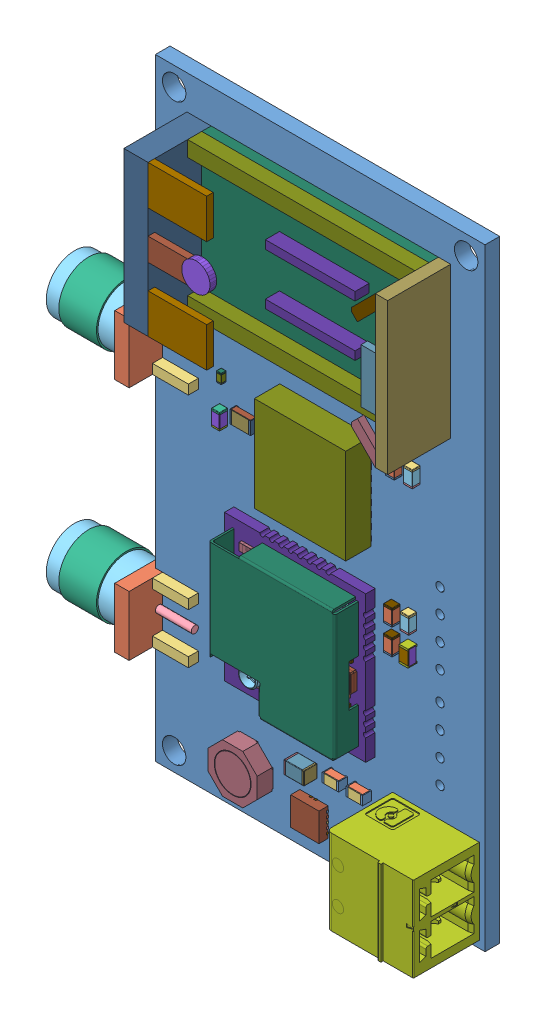
SolidWorks assembly Peggy Tracker, configuration По умолчанию. Lengths in mm.
Overall size (43.58 65 10.65).
318 component instances, 80 part files, 0 mates.
Components (placement in the parent):
- Peggy Tracker.step-1: Peggy Tracker.step [Default] at origin size (43.58 65 10.65)
  - Board.step-1: Board.step [Default] at origin size (35 65 1.56)
    - Open CASCADE STEP translator 6.8 1.1.1.step-1: Open CASCADE STEP translator 6.8 1.1.1.step [Default] at (0 0 -1.5596) size (35 65 1.56)
  - XS2.step-1: XS2.step [Default] at origin size (13.15 6.35 6.72)
    - 6208988928.step-1: 6208988928.step [Default] at (0 14.605 -2.8) size (1.52 6.35 6.35)
      - Extruded.step-1: Extruded.step [Default] at origin size (1.52 6.35 6.35)
    - 6208988528.step-1: 6208988528.step [Default] at (2.667 11.938 0) size (3.81 1.02 1.07)
      - Extruded-0.step-1: Extruded-0.step [Default] at origin size (3.81 1.02 1.07)
    - 6208988528.step-2: 6208988528.step [Default] at (2.667 17.272 0) size (3.81 1.02 1.07)
      - Extruded-0.step-1: Extruded-0.step [Default] at origin size (3.81 1.02 1.07)
    - 6208987888.step-1: 6208987888.step [Default] at (0.7603 14.6035 0.38) x (0 1 0) z (1 0 0) size (0.76 0.76 3.81)
      - Cylinder.step-1: Cylinder.step [Default] at origin size (0.76 0.76 3.81)
    - 6208988528.step-3: 6208988528.step [Default] at (2.667 11.938 -2.8) size (3.81 1.02 1.07)
      - Extruded-0.step-1: Extruded-0.step [Default] at origin size (3.81 1.02 1.07)
    - 6208988528.step-4: 6208988528.step [Default] at (2.667 17.272 -2.8) size (3.81 1.02 1.07)
      - Extruded-0.step-1: Extruded-0.step [Default] at origin size (3.81 1.02 1.07)
    - 6208987088.step-1: 6208987088.step [Default] at (-8.58 14.6049 0) x (0 1 0) z (1 0 0) size (6 6 7.87)
      - Cylinder-1.step-1: Cylinder-1.step [Default] at origin size (6 6 7.87)
    - 6208986608.step-1: 6208986608.step [Default] at (-7.0799 14.6099 0) x (0 1 0) z (1 0 0) size (6.34 6.34 4)
      - Cylinder-2.step-1: Cylinder-2.step [Default] at origin size (6.34 6.34 4)
  - XS1.step-1: XS1.step [Default] at origin size (13.15 6.35 6.72)
    - 6208986608.step-1: 6208986608.step [Default] at (-7.0799 39.6797 0) x (0 1 0) z (1 0 0) size (6.34 6.34 4)
      - Cylinder-2.step-1: Cylinder-2.step [Default] at origin size (6.34 6.34 4)
    - 6208987088.step-1: 6208987088.step [Default] at (-8.58 39.6747 0) x (0 1 0) z (1 0 0) size (6 6 7.87)
      - Cylinder-1.step-1: Cylinder-1.step [Default] at origin size (6 6 7.87)
    - 6208988528.step-1: 6208988528.step [Default] at (2.667 42.3418 -2.8) size (3.81 1.02 1.07)
      - Extruded-0.step-1: Extruded-0.step [Default] at origin size (3.81 1.02 1.07)
    - 6208988528.step-2: 6208988528.step [Default] at (2.667 37.0078 -2.8) size (3.81 1.02 1.07)
      - Extruded-0.step-1: Extruded-0.step [Default] at origin size (3.81 1.02 1.07)
    - 6208987888.step-1: 6208987888.step [Default] at (0.7603 39.6733 0.38) x (0 1 0) z (1 0 0) size (0.76 0.76 3.81)
      - Cylinder.step-1: Cylinder.step [Default] at origin size (0.76 0.76 3.81)
    - 6208988528.step-3: 6208988528.step [Default] at (2.667 42.3418 0) size (3.81 1.02 1.07)
      - Extruded-0.step-1: Extruded-0.step [Default] at origin size (3.81 1.02 1.07)
    - 6208988528.step-4: 6208988528.step [Default] at (2.667 37.0078 0) size (3.81 1.02 1.07)
      - Extruded-0.step-1: Extruded-0.step [Default] at origin size (3.81 1.02 1.07)
    - 6208988928.step-1: 6208988928.step [Default] at (0 39.6748 -2.8) size (1.52 6.35 6.35)
      - Extruded.step-1: Extruded.step [Default] at origin size (1.52 6.35 6.35)
  - X3.step-1: X3.step [Default] at origin size (9.3 9.01 10.65)
    - 1803277.step-1: 1803277.step [Default] at (25.1905 3.3527 0) x (1 0 0) z (0 -1 0) size (9.3 10.65 9.01)
  - X1.step-1: X1.step [Default] at origin size (28 16 6.7)
    - 6208991008.step-1: 6208991008.step [Default] at (11.004 53.3908 6) size (3 3 0.7)
      - Extruded-3.step-1: Extruded-3.step [Default] at origin size (3 3 0.7)
    - 6208986048.step-1: 6208986048.step [Default] at (9.0355 47.4853 6) size (6.22 4.19 0.7)
      - Extruded-4.step-1: Extruded-4.step [Default] at origin size (6.22 4.19 0.7)
    - 6208986048.step-2: 6208986048.step [Default] at (9.0355 59.2953 6) size (6.22 4.19 0.7)
      - Extruded-4.step-1: Extruded-4.step [Default] at origin size (6.22 4.19 0.7)
    - 6208985488.step-1: 6208985488.step [Default] at (4.639 53.3903 0) size (2.57 16 6.7)
      - Extruded-5.step-1: Extruded-5.step [Default] at origin size (2.57 16 6.7)
    - 6208985328.step-1: 6208985328.step [Default] at (8.0358 53.4043 6) size (4.22 2.41 0.7)
      - Extruded-6.step-1: Extruded-6.step [Default] at origin size (4.22 2.41 0.7)
    - 6208984928.step-1: 6208984928.step [Default] at (30.7032 53.3903 0) size (1.3 16 6.7)
      - Extruded-7.step-1: Extruded-7.step [Default] at origin size (1.3 16 6.7)
    - 6208984448.step-1: 6208984448.step [Default] at (28.7845 47.1665 6) size (2.54 3.55 0.7)
      - Extruded-8.step-1: Extruded-8.step [Default] at origin size (2.54 3.55 0.7)
    - 6208984128.step-1: 6208984128.step [Default] at (29.2922 53.0733 6) size (1.52 5.71 0.7)
      - Extruded-9.step-1: Extruded-9.step [Default] at origin size (1.52 5.71 0.7)
    - 6208983808.step-1: 6208983808.step [Default] at (17.9894 53.3903 0) size (24.13 16 1)
      - Extruded-10.step-1: Extruded-10.step [Default] at origin size (24.13 16 1)
    - 6208983328.step-1: 6208983328.step [Default] at (17.989 60.5658 0) size (24.13 1.65 2.5)
      - Extruded-11.step-1: Extruded-11.step [Default] at origin size (24.13 1.65 2.5)
    - 6208983328.step-2: 6208983328.step [Default] at (17.9896 46.2145 0) size (24.13 1.65 2.5)
      - Extruded-11.step-1: Extruded-11.step [Default] at origin size (24.13 1.65 2.5)
    - 6208989168.step-1: 6208989168.step [Default] at (18.9415 50.4071 0) size (9.53 0.89 2.5)
      - Extruded-12.step-1: Extruded-12.step [Default] at origin size (9.53 0.89 2.5)
    - 6208989168.step-2: 6208989168.step [Default] at (18.9415 55.8681 0) size (9.53 0.89 2.5)
      - Extruded-12.step-1: Extruded-12.step [Default] at origin size (9.53 0.89 2.5)
    - 6208982368.step-1: 6208982368.step [Default] at (28.7842 59.6128 6) size (2.54 3.55 0.7)
      - Extruded-13.step-1: Extruded-13.step [Default] at origin size (2.54 3.55 0.7)
  - R5.step-1: R5.step [Default] at origin size (1.75 0.95 0.95)
    - 6200588496.step-1: 6200588496.step [Default] at (19.5326 8.3312 0) x (1 0 0) z (0 0 1) size (1.75 0.95 0.95)
      - Terminal.step-1: Terminal.step [Default] at (-0.875 -0.475 0) size (0.2 0.95 0.95)
        - Open_CASCADE_STEP_translator_6.8_12.2.1.step-1: Open_CASCADE_STEP_translator_6.8_12.2.1.step [Default] at origin size (0.2 0.95 0.95)
      - Terminal.step-2: Terminal.step [Default] at (0.875 0.475 0) x (-1 0 0) z (0 0 1) size (0.2 0.95 0.95)
        - Open_CASCADE_STEP_translator_6.8_12.2.1.step-1: Open_CASCADE_STEP_translator_6.8_12.2.1.step [Default] at origin size (0.2 0.95 0.95)
      - Mid_Body.step-1: Mid_Body.step [Default] at (-0.875 -0.475 0) size (1.56 0.95 0.76)
      - Mark.step-1: Mark.step [Default] at (-0.675 -0.475 0.855) size (1.35 0.95 0.1)
  - R4.step-1: R4.step [Default] at origin size (1.75 0.95 0.95)
    - 6200588496.step-1: 6200588496.step [Default] at (22.0726 8.3312 0) x (1 0 0) z (0 0 1) size (1.75 0.95 0.95)
      - Terminal.step-1: Terminal.step [Default] at (-0.875 -0.475 0) size (0.2 0.95 0.95)
        - Open_CASCADE_STEP_translator_6.8_12.2.1.step-1: Open_CASCADE_STEP_translator_6.8_12.2.1.step [Default] at origin size (0.2 0.95 0.95)
      - Terminal.step-2: Terminal.step [Default] at (0.875 0.475 0) x (-1 0 0) z (0 0 1) size (0.2 0.95 0.95)
        - Open_CASCADE_STEP_translator_6.8_12.2.1.step-1: Open_CASCADE_STEP_translator_6.8_12.2.1.step [Default] at origin size (0.2 0.95 0.95)
      - Mid_Body.step-1: Mid_Body.step [Default] at (-0.875 -0.475 0) size (1.56 0.95 0.76)
      - Mark.step-1: Mark.step [Default] at (-0.675 -0.475 0.855) size (1.35 0.95 0.1)
  - R3.step-1: R3.step [Default] at origin size (0.9 1.7 0.55)
    - 6200580176.step-1: 6200580176.step [Default] at (20.9551 23.2561 -1.5596) x (0 1 0) z (0 0 -1) size (1.7 0.9 0.55)
      - Terminal-1.step-1: Terminal-1.step [Default] at (-0.85 -0.45 0) size (0.1 0.9 0.55)
        - Open_CASCADE_STEP_translator_6.8_15.2.1.step-1: Open_CASCADE_STEP_translator_6.8_15.2.1.step [Default] at origin size (0.1 0.9 0.55)
      - Terminal-1.step-2: Terminal-1.step [Default] at (0.85 0.45 0) x (-1 0 0) z (0 0 1) size (0.1 0.9 0.55)
        - Open_CASCADE_STEP_translator_6.8_15.2.1.step-1: Open_CASCADE_STEP_translator_6.8_15.2.1.step [Default] at origin size (0.1 0.9 0.55)
      - Mid_Body-14.step-1: Mid_Body-14.step [Default] at (-0.85 -0.45 0) size (1.59 0.9 0.44)
      - Mark-15.step-1: Mark-15.step [Default] at (-0.75 -0.45 0.495) size (1.5 0.9 0.06)
  - R2.step-1: R2.step [Default] at origin size (0.95 1.75 0.95)
    - 6200574256.step-1: 6200574256.step [Default] at (27.3 23.8 0) x (0 1 0) z (0 0 1) size (1.75 0.95 0.95)
      - Terminal-2.step-1: Terminal-2.step [Default] at (-0.875 -0.475 0) size (0.2 0.95 0.95)
        - Open_CASCADE_STEP_translator_6.8_12.2.1-16.step-1: Open_CASCADE_STEP_translator_6.8_12.2.1-16.step [Default] at origin size (0.2 0.95 0.95)
      - Terminal-2.step-2: Terminal-2.step [Default] at (0.875 0.475 0) x (-1 0 0) z (0 0 1) size (0.2 0.95 0.95)
        - Open_CASCADE_STEP_translator_6.8_12.2.1-16.step-1: Open_CASCADE_STEP_translator_6.8_12.2.1-16.step [Default] at origin size (0.2 0.95 0.95)
      - Mid_Body-17.step-1: Mid_Body-17.step [Default] at (-0.875 -0.475 0) size (1.56 0.95 0.76)
      - Mark-18.step-1: Mark-18.step [Default] at (-0.675 -0.475 0.855) size (1.35 0.95 0.1)
  - R1.step-1: R1.step [Default] at origin size (2.2 1.35 0.7)
    - 6200587536.step-1: 6200587536.step [Default] at (9.7028 36.3728 0) size (2.2 1.35 0.7)
      - Terminal-3.step-1: Terminal-3.step [Default] at (-1.1 -0.675 0) size (0.2 1.35 0.7)
        - Open_CASCADE_STEP_translator_6.8_14.2.1.step-1: Open_CASCADE_STEP_translator_6.8_14.2.1.step [Default] at origin size (0.2 1.35 0.7)
      - Terminal-3.step-2: Terminal-3.step [Default] at (1.1 0.675 0) x (-1 0 0) z (0 0 1) size (0.2 1.35 0.7)
        - Open_CASCADE_STEP_translator_6.8_14.2.1.step-1: Open_CASCADE_STEP_translator_6.8_14.2.1.step [Default] at origin size (0.2 1.35 0.7)
      - Mid_Body-19.step-1: Mid_Body-19.step [Default] at (-1.1 -0.675 0) size (2.06 1.35 0.56)
      - Mark-20.step-1: Mark-20.step [Default] at (-0.9 -0.675 0.63) size (1.8 1.35 0.07)
  - L2.step-1: L2.step [Default] at origin size (5.2 5.2 1.8)
    - 6200580336.step-1: 6200580336.step [Default] at (10.0076 4.7622 0.2) x (0 -1 0) z (-1 0 0) size (5.2 1.8 5.2)
  - L1.step-1: L1.step [Default] at origin size (0.55 1.05 0.55)
    - 6200588576.step-1: 6200588576.step [Default] at (7.2644 39.1682 0) x (0 1 0) z (0 0 1) size (1.05 0.55 0.55)
      - Terminal-4.step-1: Terminal-4.step [Default] at (-0.525 -0.275 0) size (1.05 0.55 0.55)
        - Open_CASCADE_STEP_translator_6.8_5.1.1.step-1: Open_CASCADE_STEP_translator_6.8_5.1.1.step [Default] at origin size (0.15 0.55 0.55)
        - Open_CASCADE_STEP_translator_6.8_5.1.2.step-1: Open_CASCADE_STEP_translator_6.8_5.1.2.step [Default] at origin size (0.15 0.55 0.55)
      - Mid_Body-21.step-1: Mid_Body-21.step [Default] at (-0.525 -0.275 0) size (0.75 0.55 0.55)
        - Open_CASCADE_STEP_translator_6.8_5.2.1.step-1: Open_CASCADE_STEP_translator_6.8_5.2.1.step [Default] at origin size (0.75 0.55 0.55)
  - DD2.step-1: DD2.step [Default] at origin size (15 15.5 3.52)
    - 3D_RAK3172.step-1: 3D_RAK3172.step [Default] at (23.336 27.5721 1) x (-1 0 0) z (0 0 1) size (15 15.5 3.52)
      - Board-1.step-1: Board-1.step [Default] at origin size (15 15.5 1.01)
        - Open_CASCADE_STEP_translator_6.8_1.1.1.step-1: Open_CASCADE_STEP_translator_6.8_1.1.1.step [Default] at (0 0 -1.014) size (15 15.5 1.01)
          - Open_CASCADE_STEP_translator_6.8_1.1.1.1.step-1: Open_CASCADE_STEP_translator_6.8_1.1.1.1.step [Default] at origin size (15 15.5 1.01)
      - R11.step-1: R11.step [Default] at origin size (0.6 0.3 0.3)
        - 0201_SMD_Capacitor.step-1: 0201_SMD_Capacitor.step [Default] at (3.4751 6.9342 0.2794) x (-1 0 0) z (0 0 1) size (0.6 0.3 0.3)
      - U2.step-1: U2.step [Default] at origin size (0.99 1.02 0.75)
        - 6590464912.step-1: 6590464912.step [Default] at (5.4483 13.05 0) size (0.99 1.02 0.75)
          - Extruded-22.step-1: Extruded-22.step [Default] at origin size (0.99 1.02 0.75)
      - R4-1.step-1: R4-1.step [Default] at origin size (0.68 0.33 0.34)
        - R0201.step-1: R0201.step [Default] at (3.9176 5.9192 0) x (1 0 0) z (0 -1 0) size (0.68 0.34 0.33)
      - R3-1.step-1: R3-1.step [Default] at origin size (0.33 0.68 0.34)
        - R0201.step-1: R0201.step [Default] at (4.1676 5.6692 0) x (0 1 0) z (1 0 0) size (0.68 0.34 0.33)
      - L2-1.step-1: L2-1.step [Default] at origin size (1.15 0.55 0.41)
        - RES_1005-0402.step-1: RES_1005-0402.step [Default] at (2.2661 6.0198 0) x (1 0 0) z (0 -1 0) size (1.15 0.41 0.55)
      - C10.step-1: C10.step [Default] at origin size (0.6 0.3 0.3)
        - 0201_SMD_Capacitor.step-1: 0201_SMD_Capacitor.step [Default] at (7.1835 13.462 0.2794) x (-1 0 0) z (0 0 1) size (0.6 0.3 0.3)
      - C9.step-1: C9.step [Default] at origin size (0.6 0.3 0.3)
        - 0201_SMD_Capacitor.step-1: 0201_SMD_Capacitor.step [Default] at (7.1835 13.97 0.2794) x (-1 0 0) z (0 0 1) size (0.6 0.3 0.3)
      - C8.step-1: C8.step [Default] at origin size (0.6 0.3 0.3)
        - 0201_SMD_Capacitor.step-1: 0201_SMD_Capacitor.step [Default] at (7.1835 12.954 0.2794) x (-1 0 0) z (0 0 1) size (0.6 0.3 0.3)
      - C7.step-1: C7.step [Default] at origin size (0.6 0.3 0.3)
        - 0201_SMD_Capacitor.step-1: 0201_SMD_Capacitor.step [Default] at (6.0793 11.938 0.2794) x (1 0 0) z (0 0 1) size (0.6 0.3 0.3)
      - C6.step-1: C6.step [Default] at origin size (0.6 0.3 0.3)
        - 0201_SMD_Capacitor.step-1: 0201_SMD_Capacitor.step [Default] at (3.8855 13.5541 0.2794) x (-1 0 0) z (0 0 1) size (0.6 0.3 0.3)
      - CON1.step-1: CON1.step [Default] at origin size (3.4 3.1 1.25)
        - UFL-R-SMD.step-1: UFL-R-SMD.step [Default] at (11.3537 12.7757 0) x (1 0 0) z (0 0 1) size (3.4 3.1 1.25)
          - Part_525.step-1: Part_525.step [Default] at origin size (3 2.6 0.35)
          - Part_739.step-1: Part_739.step [Default] at origin size (2 2 0.9)
          - Part_578.step-1: Part_578.step [Default] at origin size (0.6 0.5 0.1)
          - Part_540.step-1: Part_540.step [Default] at origin size (0.4 1.8 0.1)
          - Part_562.step-1: Part_562.step [Default] at origin size (0.4 1.8 0.1)
          - Part_555.step-1: Part_555.step [Default] at origin size (0.6 0.5 0.1)
      - C4.step-1: C4.step [Default] at origin size (0.6 0.3 0.3)
        - 0201_SMD_Capacitor.step-1: 0201_SMD_Capacitor.step [Default] at (3.7799 9.398 0.2794) x (-1 0 0) z (0 0 1) size (0.6 0.3 0.3)
      - U1.step-1: U1.step [Default] at origin size (7.02 7.02 0.8)
        - QFN48_7x7.step-1: QFN48_7x7.step [Default] at (8.8366 6.9818 0) x (0 1 0) z (1 0 0) size (7.02 0.8 7.02)
      - X1-1.step-1: X1-1.step [Default] at origin size (1.61 2.01 0.71)
        - NT2016SA.step-1: NT2016SA.step [Default] at (1.7496 8.4946 0) x (0 1 0) z (1 0 0) size (2.01 0.71 1.61)
      - C43.step-1: C43.step [Default] at origin size (0.6 0.3 0.3)
        - 0201_SMD_Capacitor.step-1: 0201_SMD_Capacitor.step [Default] at (3.7799 9.9822 0.2794) x (-1 0 0) z (0 0 1) size (0.6 0.3 0.3)
      - C42.step-1: C42.step [Default] at origin size (0.3 0.6 0.3)
        - 0201_SMD_Capacitor.step-1: 0201_SMD_Capacitor.step [Default] at (3.0734 7.9709 0.2794) x (0 -1 0) z (0 0 1) size (0.6 0.3 0.3)
      - R9.step-1: R9.step [Default] at origin size (0.6 0.3 0.3)
        - 0201_SMD_Capacitor.step-1: 0201_SMD_Capacitor.step [Default] at (3.7799 8.8138 0.2794) x (-1 0 0) z (0 0 1) size (0.6 0.3 0.3)
      - C1.step-1: C1.step [Default] at origin size (0.6 0.3 0.3)
        - 0201_SMD_Capacitor.step-1: 0201_SMD_Capacitor.step [Default] at (7.0445 11.557 0.2794) x (1 0 0) z (0 0 1) size (0.6 0.3 0.3)
      - C2.step-1: C2.step [Default] at origin size (0.3 0.6 0.3)
        - 0201_SMD_Capacitor.step-1: 0201_SMD_Capacitor.step [Default] at (7.9756 12.2635 0.2794) x (0 -1 0) z (0 0 1) size (0.6 0.3 0.3)
      - C3.step-1: C3.step [Default] at origin size (0.3 0.6 0.3)
        - 0201_SMD_Capacitor.step-1: 0201_SMD_Capacitor.step [Default] at (2.1844 13.4518 0.2794) x (0 -1 0) z (0 0 1) size (0.6 0.3 0.3)
      - C11.step-1: C11.step [Default] at origin size (0.6 0.3 0.3)
        - 0201_SMD_Capacitor.step-1: 0201_SMD_Capacitor.step [Default] at (1.6623 11.9866 0.2794) x (1 0 0) z (0 0 1) size (0.6 0.3 0.3)
      - C12.step-1: C12.step [Default] at origin size (0.6 0.3 0.3)
        - 0201_SMD_Capacitor.step-1: 0201_SMD_Capacitor.step [Default] at (3.2813 12.573 0.2794) x (1 0 0) z (0 0 1) size (0.6 0.3 0.3)
      - C13.step-1: C13.step [Default] at origin size (0.3 0.6 0.3)
        - 0201_SMD_Capacitor.step-1: 0201_SMD_Capacitor.step [Default] at (4.4958 12.0697 0.2794) x (0 1 0) z (0 0 1) size (0.6 0.3 0.3)
      - C14.step-1: C14.step [Default] at origin size (0.3 0.6 0.3)
        - 0201_SMD_Capacitor.step-1: 0201_SMD_Capacitor.step [Default] at (2.7178 12.6739 0.2794) x (0 -1 0) z (0 0 1) size (0.6 0.3 0.3)
      - C17.step-1: C17.step [Default] at origin size (0.3 0.6 0.3)
        - 0201_SMD_Capacitor.step-1: 0201_SMD_Capacitor.step [Default] at (7.6708 14.4693 0.2794) x (0 -1 0) z (0 0 1) size (0.6 0.3 0.3)
      - C18.step-1: C18.step [Default] at origin size (0.6 0.3 0.3)
        - 0201_SMD_Capacitor.step-1: 0201_SMD_Capacitor.step [Default] at (9.1901 14.1224 0.2794) x (-1 0 0) z (0 0 1) size (0.6 0.3 0.3)
      - C19.step-1: C19.step [Default] at origin size (0.3 0.6 0.3)
        - 0201_SMD_Capacitor.step-1: 0201_SMD_Capacitor.step [Default] at (2.8814 10.8799 0.2794) x (0 1 0) z (0 0 1) size (0.6 0.3 0.3)
      - C22.step-1: C22.step [Default] at origin size (0.3 0.6 0.3)
        - 0201_SMD_Capacitor.step-1: 0201_SMD_Capacitor.step [Default] at (2.0432 11.4801 0.2794) x (0 -1 0) z (0 0 1) size (0.6 0.3 0.3)
      - C21.step-1: C21.step [Default] at origin size (0.3 0.6 0.3)
        - 0201_SMD_Capacitor.step-1: 0201_SMD_Capacitor.step [Default] at (1.5606 11.4801 0.2794) x (0 -1 0) z (0 0 1) size (0.6 0.3 0.3)
      - C23.step-1: C23.step [Default] at origin size (1 0.5 0.5)
        - C0402.step-1: C0402.step [Default] at (8.9644 1.5539 0.254) x (1 0 0) z (0 0 1) size (1 0.5 0.5)
      - C24.step-1: C24.step [Default] at origin size (0.6 0.3 0.3)
        - 0201_SMD_Capacitor.step-1: 0201_SMD_Capacitor.step [Default] at (4.7197 3.8862 0.2794) x (-1 0 0) z (0 0 1) size (0.6 0.3 0.3)
      - C26.step-1: C26.step [Default] at origin size (0.3 0.6 0.3)
        - 0201_SMD_Capacitor.step-1: 0201_SMD_Capacitor.step [Default] at (10.541 2.2265 0.2794) x (0 -1 0) z (0 0 1) size (0.6 0.3 0.3)
      - C44.step-1: C44.step [Default] at origin size (0.6 0.3 0.3)
        - 0201_SMD_Capacitor.step-1: 0201_SMD_Capacitor.step [Default] at (4.7919 9.9822 0.2794) x (-1 0 0) z (0 0 1) size (0.6 0.3 0.3)
      - C29.step-1: C29.step [Default] at origin size (0.6 0.3 0.3)
        - 0201_SMD_Capacitor.step-1: 0201_SMD_Capacitor.step [Default] at (3.9925 7.8486 0.2794) x (1 0 0) z (0 0 1) size (0.6 0.3 0.3)
      - C25.step-1: C25.step [Default] at origin size (0.3 0.6 0.3)
        - 0201_SMD_Capacitor.step-1: 0201_SMD_Capacitor.step [Default] at (10.287 1.6263 0.2794) x (0 1 0) z (0 0 1) size (0.6 0.3 0.3)
      - C31.step-1: C31.step [Default] at origin size (0.6 0.3 0.3)
        - 0201_SMD_Capacitor.step-1: 0201_SMD_Capacitor.step [Default] at (3.9965 7.239 0.2794) x (1 0 0) z (0 0 1) size (0.6 0.3 0.3)
      - C32.step-1: C32.step [Default] at origin size (0.6 0.3 0.3)
        - 0201_SMD_Capacitor.step-1: 0201_SMD_Capacitor.step [Default] at (7.8533 2.3622 0.2794) x (1 0 0) z (0 0 1) size (0.6 0.3 0.3)
      - C33.step-1: C33.step [Default] at origin size (1 0.5 0.5)
        - C0402.step-1: C0402.step [Default] at (5.3048 2.0461 0.254) x (-1 0 0) z (0 0 1) size (1 0.5 0.5)
      - C34.step-1: C34.step [Default] at origin size (0.3 0.6 0.3)
        - 0201_SMD_Capacitor.step-1: 0201_SMD_Capacitor.step [Default] at (4.318 4.2211 0.2794) x (0 1 0) z (0 0 1) size (0.6 0.3 0.3)
      - C35.step-1: C35.step [Default] at origin size (0.6 0.3 0.3)
        - 0201_SMD_Capacitor.step-1: 0201_SMD_Capacitor.step [Default] at (9.0365 2.3622 0.2794) x (1 0 0) z (0 0 1) size (0.6 0.3 0.3)
      - C36.step-1: C36.step [Default] at origin size (0.3 0.6 0.3)
        - 0201_SMD_Capacitor.step-1: 0201_SMD_Capacitor.step [Default] at (13.0302 10.0751 0.2794) x (0 -1 0) z (0 0 1) size (0.6 0.3 0.3)
      - C37.step-1: C37.step [Default] at origin size (0.3 0.6 0.3)
        - 0201_SMD_Capacitor.step-1: 0201_SMD_Capacitor.step [Default] at (3.7338 4.2211 0.2794) x (0 1 0) z (0 0 1) size (0.6 0.3 0.3)
      - C38.step-1: C38.step [Default] at origin size (1 0.5 0.5)
        - C0402.step-1: C0402.step [Default] at (2.3114 4.7323 0.254) x (1 0 0) z (0 0 1) size (1 0.5 0.5)
      - C39.step-1: C39.step [Default] at origin size (0.6 0.3 0.3)
        - 0201_SMD_Capacitor.step-1: 0201_SMD_Capacitor.step [Default] at (4.0593 3.1881 0.2794) x (-1 0 0) z (0 0 1) size (0.6 0.3 0.3)
      - C40.step-1: C40.step [Default] at origin size (0.3 0.6 0.3)
        - 0201_SMD_Capacitor.step-1: 0201_SMD_Capacitor.step [Default] at (3.6576 1.7319 0.2794) x (0 1 0) z (0 0 1) size (0.6 0.3 0.3)
      - L1-1.step-1: L1-1.step [Default] at origin size (0.68 0.33 0.34)
        - R0201.step-1: R0201.step [Default] at (7.8526 11.2014 0) x (-1 0 0) z (0 1 0) size (0.68 0.34 0.33)
      - L3.step-1: L3.step [Default] at origin size (0.33 0.68 0.34)
        - R0201.step-1: R0201.step [Default] at (1.7272 13.1318 0) x (0 -1 0) z (-1 0 0) size (0.68 0.34 0.33)
      - L5.step-1: L5.step [Default] at origin size (0.68 0.33 0.34)
        - R0201.step-1: R0201.step [Default] at (8.0772 13.3096 0) x (-1 0 0) z (0 1 0) size (0.68 0.34 0.33)
      - L6.step-1: L6.step [Default] at origin size (1 0.5 0.5)
        - C0402.step-1: C0402.step [Default] at (5.822 11.0823 0.254) x (1 0 0) z (0 0 1) size (1 0.5 0.5)
      - L7.step-1: L7.step [Default] at origin size (0.68 0.33 0.34)
        - R0201.step-1: R0201.step [Default] at (3.5854 12.1158 0) x (1 0 0) z (0 -1 0) size (0.68 0.34 0.33)
      - L9.step-1: L9.step [Default] at origin size (1.15 0.55 0.41)
        - RES_1005-0402.step-1: RES_1005-0402.step [Default] at (3.9641 11.3538 0) x (-1 0 0) z (0 1 0) size (1.15 0.41 0.55)
      - L20.step-1: L20.step [Default] at origin size (1.6 0.8 0.3)
        - 6559637360.step-1: 6559637360.step [Default] at (12.3698 2.0828 0) x (-1 0 0) z (0 1 0) size (1.6 0.3 0.8)
      - L30.step-1: L30.step [Default] at origin size (1.15 0.55 0.41)
        - RES_1005-0402.step-1: RES_1005-0402.step [Default] at (7.1263 1.8 0) x (-1 0 0) z (0 1 0) size (1.15 0.41 0.55)
      - X2.step-1: X2.step [Default] at origin size (1.2 2 0.61)
        - crystal_rtf2012.step-1: crystal_rtf2012.step [Default] at (2.25 2.8402 0) x (0 1 0) z (1 0 0) size (2 0.61 1.2)
      - R2-1.step-1: R2-1.step [Default] at origin size (0.68 0.33 0.34)
        - R0201.step-1: R0201.step [Default] at (1.9613 10.1854 0) x (1 0 0) z (0 -1 0) size (0.68 0.34 0.33)
      - C5.step-1: C5.step [Default] at origin size (0.6 0.3 0.3)
        - 0201_SMD_Capacitor.step-1: 0201_SMD_Capacitor.step [Default] at (1.8749 6.9342 0.2794) x (-1 0 0) z (0 0 1) size (0.6 0.3 0.3)
      - Free-Models.step-1: Free-Models.step [Default] at origin size (13.4 13.9 2.5)
        - D030A-______.step-1: D030A-______.step [Default] at (2.429 -1.8288 0) size (13.4 13.9 2.5)
  - DD1.step-1: DD1.step [Default] at origin size (9.7 10.1 2.8)
    - 6200574736.step-1: 6200574736.step [Default] at (18.161 36.3728 0) x (1 0 0) z (0 0 1) size (9.7 10.1 2.8)
      - Body.step-1: Body.step [Default] at (0 0 0.1) size (9.7 10.1 2.7)
      - Pins.step-1: Pins.step [Default] at origin size (9.56 9.36 0.1)
  - DA1.step-1: DA1.step [Default] at origin size (3 3 1)
    - 6200580816.step-1: 6200580816.step [Default] at (16.8686 3.6162 0) x (1 0 0) z (0 0 1) size (3 3 1)
      - FRAME-DRC0010J.step-1: FRAME-DRC0010J.step [Default] x (1 0 0) z (0 -1 0) size (3 0.2 3)
        - Open CASCADE STEP translator 6.8 1.15.1.2.1.step-1: Open CASCADE STEP translator 6.8 1.15.1.2.1.step [Default] at origin size (1.9 0.2 3)
        - Open CASCADE STEP translator 6.8 1.15.1.2.2.step-1: Open CASCADE STEP translator 6.8 1.15.1.2.2.step [Default] at origin size (0.4 0.2 0.24)
        - Open CASCADE STEP translator 6.8 1.15.1.2.3.step-1: Open CASCADE STEP translator 6.8 1.15.1.2.3.step [Default] at origin size (0.4 0.2 0.24)
        - Open CASCADE STEP translator 6.8 1.15.1.2.4.step-1: Open CASCADE STEP translator 6.8 1.15.1.2.4.step [Default] at origin size (0.4 0.2 0.24)
        - Open CASCADE STEP translator 6.8 1.15.1.2.5.step-1: Open CASCADE STEP translator 6.8 1.15.1.2.5.step [Default] at origin size (0.4 0.2 0.24)
        - Open CASCADE STEP translator 6.8 1.15.1.2.6.step-1: Open CASCADE STEP translator 6.8 1.15.1.2.6.step [Default] at origin size (0.4 0.2 0.24)
        - Open CASCADE STEP translator 6.8 1.15.1.2.7.step-1: Open CASCADE STEP translator 6.8 1.15.1.2.7.step [Default] at origin size (0.4 0.2 0.24)
        - Open CASCADE STEP translator 6.8 1.15.1.2.8.step-1: Open CASCADE STEP translator 6.8 1.15.1.2.8.step [Default] at origin size (0.4 0.2 0.24)
        - Open CASCADE STEP translator 6.8 1.15.1.2.9.step-1: Open CASCADE STEP translator 6.8 1.15.1.2.9.step [Default] at origin size (0.4 0.2 0.24)
        - Open CASCADE STEP translator 6.8 1.15.1.2.10.step-1: Open CASCADE STEP translator 6.8 1.15.1.2.10.step [Default] at origin size (0.4 0.2 0.24)
        - Open CASCADE STEP translator 6.8 1.15.1.2.11.step-1: Open CASCADE STEP translator 6.8 1.15.1.2.11.step [Default] at origin size (0.4 0.2 0.24)
      - BODY-SON.step-1: BODY-SON.step [Default] at (0 0 0.025) x (1 0 0) z (0 -1 0) size (3 0.97 3)
  - C8-1.step-1: C8-1.step [Default] at origin size (2.15 1.4 1.4)
    - 6200588096.step-1: 6200588096.step [Default] at (16.1035 7.6961 0) x (-1 0 0) z (0 0 1) size (2.15 1.4 1.4)
      - Terminal-5.step-1: Terminal-5.step [Default] at (-1.075 -0.7 0) size (2.15 1.4 1.4)
        - Open_CASCADE_STEP_translator_6.8_5.1.1-23.step-1: Open_CASCADE_STEP_translator_6.8_5.1.1-23.step [Default] at origin size (0.2 1.4 1.4)
        - Open_CASCADE_STEP_translator_6.8_5.1.2-24.step-1: Open_CASCADE_STEP_translator_6.8_5.1.2-24.step [Default] at origin size (0.2 1.4 1.4)
      - Mid_Body-1.step-1: Mid_Body-1.step [Default] at (-1.075 -0.7 0) size (1.75 1.4 1.4)
        - Open_CASCADE_STEP_translator_6.8_5.2.1-25.step-1: Open_CASCADE_STEP_translator_6.8_5.2.1-25.step [Default] at origin size (1.75 1.4 1.4)
  - C7-1.step-1: C7-1.step [Default] at origin size (1.9 3.5 1.9)
    - 6200579696.step-1: 6200579696.step [Default] at (22.8854 3.683 0) x (0 -1 0) z (0 0 1) size (3.5 1.9 1.9)
      - Terminal-6.step-1: Terminal-6.step [Default] at (-1.75 -0.95 0) size (3.5 1.9 1.9)
        - Open_CASCADE_STEP_translator_6.8_20.1.1.step-1: Open_CASCADE_STEP_translator_6.8_20.1.1.step [Default] at origin size (0.3 1.9 1.9)
        - Open_CASCADE_STEP_translator_6.8_20.1.2.step-1: Open_CASCADE_STEP_translator_6.8_20.1.2.step [Default] at origin size (0.3 1.9 1.9)
      - Mid_Body-2.step-1: Mid_Body-2.step [Default] at (-1.75 -0.95 0) size (2.9 1.9 1.9)
        - Open_CASCADE_STEP_translator_6.8_20.2.1.step-1: Open_CASCADE_STEP_translator_6.8_20.2.1.step [Default] at origin size (2.9 1.9 1.9)
  - C6-1.step-1: C6-1.step [Default] at origin size (0.95 1.75 0.87)
    - 6200577296.step-1: 6200577296.step [Default] at (25.527 23.875 0) x (0 -1 0) z (0 0 1) size (1.75 0.95 0.87)
      - Terminal-7.step-1: Terminal-7.step [Default] at (-0.875 -0.475 0) size (1.75 0.95 0.87)
        - Open_CASCADE_STEP_translator_6.8_128.1.1.step-1: Open_CASCADE_STEP_translator_6.8_128.1.1.step [Default] at origin size (0.2 0.95 0.87)
        - Open_CASCADE_STEP_translator_6.8_128.1.2.step-1: Open_CASCADE_STEP_translator_6.8_128.1.2.step [Default] at origin size (0.2 0.95 0.87)
      - Mid_Body-3.step-1: Mid_Body-3.step [Default] at (-0.875 -0.475 0) size (1.35 0.95 0.87)
        - Open_CASCADE_STEP_translator_6.8_128.2.1.step-1: Open_CASCADE_STEP_translator_6.8_128.2.1.step [Default] at origin size (1.35 0.95 0.87)
  - C5-1.step-1: C5-1.step [Default] at origin size (0.95 1.75 0.87)
    - 6200574176.step-1: 6200574176.step [Default] at (27.305 26.76 0) x (0 -1 0) z (0 0 1) size (1.75 0.95 0.87)
      - Terminal-8.step-1: Terminal-8.step [Default] at (-0.875 -0.475 0) size (1.75 0.95 0.87)
        - Open_CASCADE_STEP_translator_6.8_129.1.1.step-1: Open_CASCADE_STEP_translator_6.8_129.1.1.step [Default] at origin size (0.2 0.95 0.87)
        - Open_CASCADE_STEP_translator_6.8_129.1.2.step-1: Open_CASCADE_STEP_translator_6.8_129.1.2.step [Default] at origin size (0.2 0.95 0.87)
      - Mid_Body-4.step-1: Mid_Body-4.step [Default] at (-0.875 -0.475 0) size (1.35 0.95 0.87)
        - Open_CASCADE_STEP_translator_6.8_129.2.1.step-1: Open_CASCADE_STEP_translator_6.8_129.2.1.step [Default] at origin size (1.35 0.95 0.87)
  - C4-1.step-1: C4-1.step [Default] at origin size (0.95 1.75 0.87)
    - 6200577296.step-1: 6200577296.step [Default] at (25.527 26.61 0) x (0 -1 0) z (0 0 1) size (1.75 0.95 0.87)
      - Terminal-7.step-1: Terminal-7.step [Default] at (-0.875 -0.475 0) size (1.75 0.95 0.87)
        - Open_CASCADE_STEP_translator_6.8_128.1.1.step-1: Open_CASCADE_STEP_translator_6.8_128.1.1.step [Default] at origin size (0.2 0.95 0.87)
        - Open_CASCADE_STEP_translator_6.8_128.1.2.step-1: Open_CASCADE_STEP_translator_6.8_128.1.2.step [Default] at origin size (0.2 0.95 0.87)
      - Mid_Body-3.step-1: Mid_Body-3.step [Default] at (-0.875 -0.475 0) size (1.35 0.95 0.87)
        - Open_CASCADE_STEP_translator_6.8_128.2.1.step-1: Open_CASCADE_STEP_translator_6.8_128.2.1.step [Default] at origin size (1.35 0.95 0.87)
  - C3-1.step-1: C3-1.step [Default] at origin size (0.95 1.75 0.87)
    - 6200574176.step-1: 6200574176.step [Default] at (27.6606 40.3998 0) x (0 -1 0) z (0 0 1) size (1.75 0.95 0.87)
      - Terminal-8.step-1: Terminal-8.step [Default] at (-0.875 -0.475 0) size (1.75 0.95 0.87)
        - Open_CASCADE_STEP_translator_6.8_129.1.1.step-1: Open_CASCADE_STEP_translator_6.8_129.1.1.step [Default] at origin size (0.2 0.95 0.87)
        - Open_CASCADE_STEP_translator_6.8_129.1.2.step-1: Open_CASCADE_STEP_translator_6.8_129.1.2.step [Default] at origin size (0.2 0.95 0.87)
      - Mid_Body-4.step-1: Mid_Body-4.step [Default] at (-0.875 -0.475 0) size (1.35 0.95 0.87)
        - Open_CASCADE_STEP_translator_6.8_129.2.1.step-1: Open_CASCADE_STEP_translator_6.8_129.2.1.step [Default] at origin size (1.35 0.95 0.87)
  - C2-1.step-1: C2-1.step [Default] at origin size (0.95 1.75 0.87)
    - 6200577296.step-1: 6200577296.step [Default] at (25.7556 40.2498 0) x (0 -1 0) z (0 0 1) size (1.75 0.95 0.87)
      - Terminal-7.step-1: Terminal-7.step [Default] at (-0.875 -0.475 0) size (1.75 0.95 0.87)
        - Open_CASCADE_STEP_translator_6.8_128.1.1.step-1: Open_CASCADE_STEP_translator_6.8_128.1.1.step [Default] at origin size (0.2 0.95 0.87)
        - Open_CASCADE_STEP_translator_6.8_128.1.2.step-1: Open_CASCADE_STEP_translator_6.8_128.1.2.step [Default] at origin size (0.2 0.95 0.87)
      - Mid_Body-3.step-1: Mid_Body-3.step [Default] at (-0.875 -0.475 0) size (1.35 0.95 0.87)
        - Open_CASCADE_STEP_translator_6.8_128.2.1.step-1: Open_CASCADE_STEP_translator_6.8_128.2.1.step [Default] at origin size (1.35 0.95 0.87)
  - C1-1.step-1: C1-1.step [Default] at origin size (0.9 1.7 0.9)
    - 6200579936.step-1: 6200579936.step [Default] at (7.2644 35.4948 0) x (0 -1 0) z (0 0 1) size (1.7 0.9 0.9)
      - Terminal-9.step-1: Terminal-9.step [Default] at (-0.85 -0.45 0) size (1.7 0.9 0.9)
        - Open_CASCADE_STEP_translator_6.8_5.1.1-26.step-1: Open_CASCADE_STEP_translator_6.8_5.1.1-26.step [Default] at origin size (0.2 0.9 0.9)
        - Open_CASCADE_STEP_translator_6.8_5.1.2-27.step-1: Open_CASCADE_STEP_translator_6.8_5.1.2-27.step [Default] at origin size (0.2 0.9 0.9)
      - Mid_Body-5.step-1: Mid_Body-5.step [Default] at (-0.85 -0.45 0) size (1.3 0.9 0.9)
        - Open_CASCADE_STEP_translator_6.8_5.2.1-28.step-1: Open_CASCADE_STEP_translator_6.8_5.2.1-28.step [Default] at origin size (1.3 0.9 0.9)
